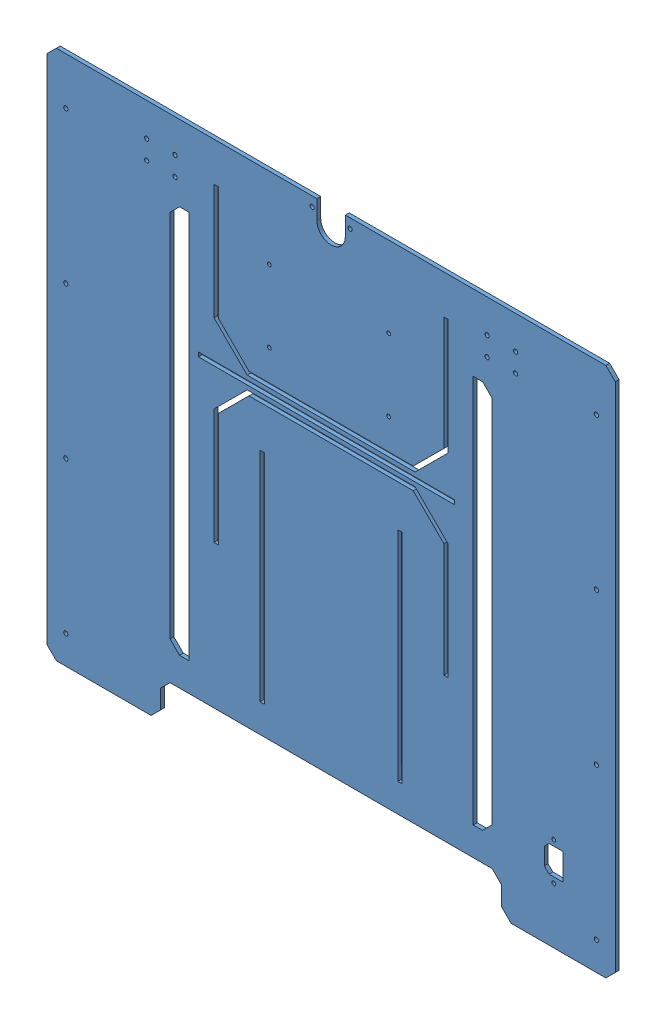
SolidWorks assembly cover_back, configuration Default. Lengths in mm.
Overall size (600 560 54.84).
3 component instances, 3 part files, 4 mates.
Components (placement in the parent):
- SheetMetal_back_cover-1: SheetMetal_back_cover [Default] at (-229.5201 169.8121 -10.2992) size (600 560 1.5)
- PSupply-1: PSupply [Default] at (30.3366 -114.7233 -63.6392) x (0 1 0) z (0 0 -1) size (234.85 114.3 53.34)
- mks-1: mks [Default] at (28.5711 145.0329 -15.2992) x (1 0 0) z (0 1 0) size (144 22.79 85)
Mates (geometry in assembly coordinates):
- Coincident1: coincident anti-aligned: plane of SheetMetal_back_cover-1 through (-229.5201 169.8121 -10.2992) normal (0 0 -1); plane of PSupply-1 through (30.3366 -114.7233 -10.2992) normal (0 0 1)
- Parallel1: parallel anti-aligned: plane of SheetMetal_back_cover-1 through (-269.2004 -251.7067 -8.7992) normal (-1 0 0); plane of PSupply-1 through (87.4866 -119.9689 -12.8392) normal (1 0 0)
- Distance1: distance = 5 mm anti-aligned: plane of mks-1 through (28.5711 145.0329 -15.2992) normal (0 0 1); plane of SheetMetal_back_cover-1 through (-229.5201 169.8121 -10.2992) normal (0 0 -1)
- Distance2: distance = 30 mm aligned: plane of mks-1 through (12.8711 104.6329 -23.2992) normal (0 -1 0); plane of SheetMetal_back_cover-1 through (30.7996 74.6329 -0.2992) normal (0 -1 0)
